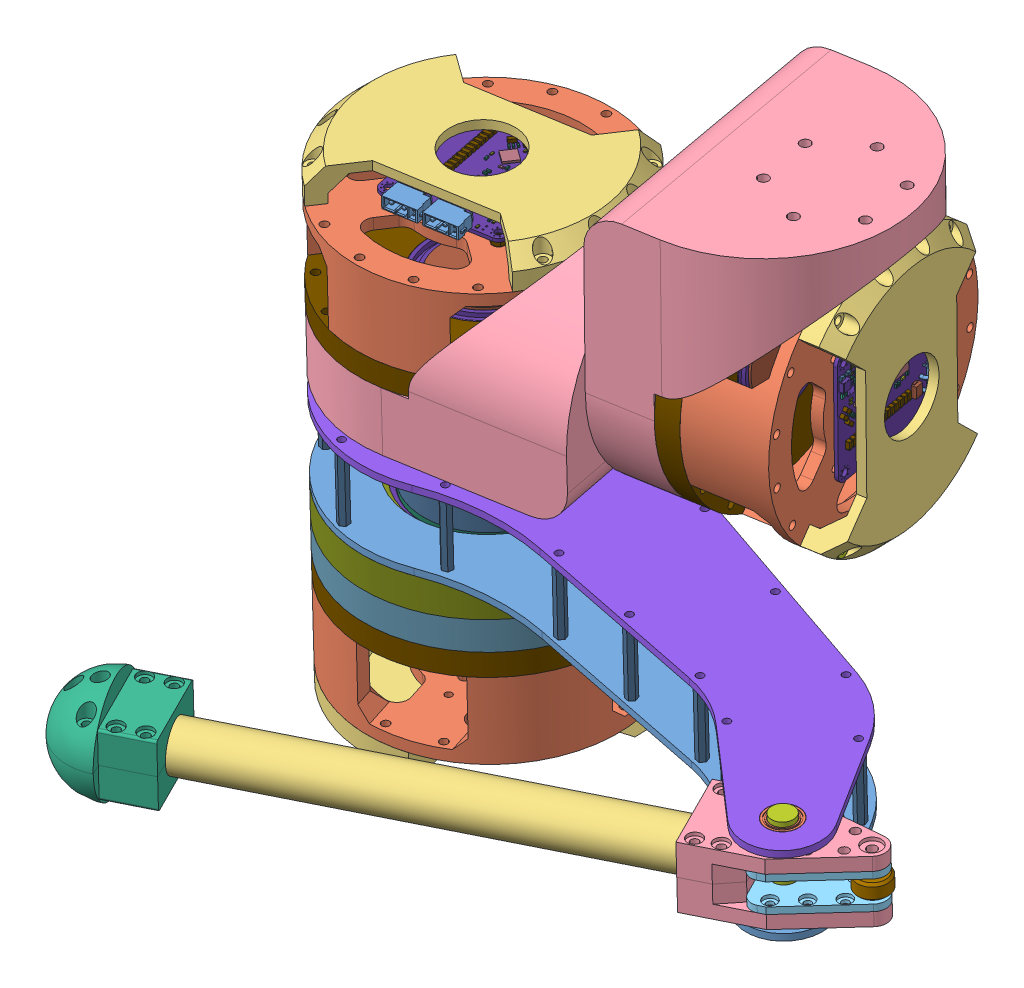
SolidWorks assembly leg, configuration Default. Lengths in mm. (continued)
Components (placement in the parent): (continued)
- Cycloidal _v3-2: Cycloidal _v3 [Default] at (218.9878 344.1312 127.6496) x (0.118839 0.702482 0.701709) z (0.116912 -0.711701 0.692685) size (173.36 87.57 173.15) (continued)
  - radial ball bearing_68_iso-46: radial ball bearing_68_iso [ISO 15 RBB - 1715 - 26,SI,NC,26_68] at (47.6295 89.6575 91.1168) x (-0.000399 1 0) z (0 0 1) size (4 21 21)
  - foc-motor-controller.step-1: foc-motor-controller.step [Default] at (47.4677 32.6574 89.6282) x (0.701413 0.00028 0.712755) z (0.000399 -1 0) size (57.23 50 8.13)
    - RTA0040B.step-1: RTA0040B.step [Default] at (12.5014 -1.6986 1.595) x (-0.707107 -0.707107 0) z (0 0 1) size (6 6 1)
      - FRAME.step-1: FRAME.step [Default] x (1 0 0) z (0 -1 0) size (6 0.2 6)
        - SOLID.step-1: SOLID.step [Default] at origin size (0.4 0.2 0.22)
        - SOLID-0.step-1: SOLID-0.step [Default] at origin size (0.4 0.2 0.22)
        - SOLID-1.step-1: SOLID-1.step [Default] at origin size (0.4 0.2 0.22)
        - SOLID-2.step-1: SOLID-2.step [Default] at origin size (0.4 0.2 0.22)
        - SOLID-3.step-1: SOLID-3.step [Default] at origin size (0.4 0.2 0.22)
        - SOLID-4.step-1: SOLID-4.step [Default] at origin size (0.4 0.2 0.22)
        - SOLID-5.step-1: SOLID-5.step [Default] at origin size (0.4 0.2 0.22)
        - SOLID-6.step-1: SOLID-6.step [Default] at origin size (0.4 0.2 0.22)
        - SOLID-7.step-1: SOLID-7.step [Default] at origin size (0.4 0.2 0.22)
        - SOLID-8.step-1: SOLID-8.step [Default] at origin size (0.4 0.2 0.22)
        - SOLID-9.step-1: SOLID-9.step [Default] at origin size (0.22 0.2 0.4)
        - SOLID-10.step-1: SOLID-10.step [Default] at origin size (0.22 0.2 0.4)
        - SOLID-11.step-1: SOLID-11.step [Default] at origin size (0.22 0.2 0.4)
        - SOLID-12.step-1: SOLID-12.step [Default] at origin size (0.22 0.2 0.4)
        - SOLID-13.step-1: SOLID-13.step [Default] at origin size (0.22 0.2 0.4)
        - SOLID-14.step-1: SOLID-14.step [Default] at origin size (0.22 0.2 0.4)
        - SOLID-15.step-1: SOLID-15.step [Default] at origin size (0.22 0.2 0.4)
        - SOLID-16.step-1: SOLID-16.step [Default] at origin size (0.22 0.2 0.4)
        - SOLID-17.step-1: SOLID-17.step [Default] at origin size (4.15 0.2 4.15)
        - SOLID-18.step-1: SOLID-18.step [Default] at origin size (0.28 0.1 0.28)
        - SOLID-19.step-1: SOLID-19.step [Default] at origin size (0.28 0.1 0.28)
        - SOLID-20.step-1: SOLID-20.step [Default] at origin size (0.28 0.1 0.28)
        - SOLID-21.step-1: SOLID-21.step [Default] at origin size (0.28 0.1 0.28)
        - SOLID-22.step-1: SOLID-22.step [Default] at origin size (0.4 0.2 0.22)
        - SOLID-23.step-1: SOLID-23.step [Default] at origin size (0.4 0.2 0.22)
        - SOLID-24.step-1: SOLID-24.step [Default] at origin size (0.4 0.2 0.22)
        - SOLID-25.step-1: SOLID-25.step [Default] at origin size (0.4 0.2 0.22)
        - SOLID-26.step-1: SOLID-26.step [Default] at origin size (0.4 0.2 0.22)
        - SOLID-27.step-1: SOLID-27.step [Default] at origin size (0.4 0.2 0.22)
        - SOLID-28.step-1: SOLID-28.step [Default] at origin size (0.4 0.2 0.22)
        - SOLID-29.step-1: SOLID-29.step [Default] at origin size (0.4 0.2 0.22)
        - SOLID-30.step-1: SOLID-30.step [Default] at origin size (0.4 0.2 0.22)
        - SOLID-31.step-1: SOLID-31.step [Default] at origin size (0.4 0.2 0.22)
        - SOLID-32.step-1: SOLID-32.step [Default] at origin size (0.22 0.2 0.4)
        - SOLID-33.step-1: SOLID-33.step [Default] at origin size (0.22 0.2 0.4)
        - SOLID-34.step-1: SOLID-34.step [Default] at origin size (0.22 0.2 0.4)
        - SOLID-35.step-1: SOLID-35.step [Default] at origin size (0.22 0.2 0.4)
        - SOLID-36.step-1: SOLID-36.step [Default] at origin size (0.22 0.2 0.4)
        - SOLID-37.step-1: SOLID-37.step [Default] at origin size (0.22 0.2 0.4)
        - SOLID-38.step-1: SOLID-38.step [Default] at origin size (0.22 0.2 0.4)
        - SOLID-39.step-1: SOLID-39.step [Default] at origin size (0.22 0.2 0.4)
        - SOLID-40.step-1: SOLID-40.step [Default] at origin size (0.22 0.2 0.4)
        - SOLID-41.step-1: SOLID-41.step [Default] at origin size (0.22 0.2 0.4)
        - SOLID-42.step-1: SOLID-42.step [Default] at origin size (0.22 0.2 0.4)
        - SOLID-43.step-1: SOLID-43.step [Default] at origin size (0.22 0.2 0.4)
      - BODY.step-1: BODY.step [Default] at (0 0 0.025) x (1 0 0) z (0 -1 0) size (6 0.97 6)
    - Resonator_SMD_Murata_CSTxExxV-3Pin_3.0x1.1mm.step-1: Resonator_SMD_Murata_CSTxExxV-3Pin_3.0x1.1mm.step [Default] at (1.8 -7 1.595) x (0 1 0) z (0 0 1) size (3.2 1.35 0.9)
    - C_0603_1608Metric.step-1: C_0603_1608Metric.step [Default] at (6.2 -16.8 1.595) x (0 -1 0) z (0 0 1) size (1.6 0.8 0.8)
    - R_0603_1608Metric.step-1: R_0603_1608Metric.step [Default] at (11.8 -7.375 1.595) x (0 1 0) z (0 0 1) size (1.6 0.8 0.45)
    - R_0603_1608Metric.step-2: R_0603_1608Metric.step [Default] at (13.8 -16.8 1.595) x (0 1 0) z (0 0 1) size (1.6 0.8 0.45)
    - R_0603_1608Metric.step-3: R_0603_1608Metric.step [Default] at (18.1 -5.36 1.595) size (1.6 0.8 0.45)
    - C_0603_1608Metric.step-2: C_0603_1608Metric.step [Default] at (2.6 -0.5 1.595) x (0 -1 0) z (0 0 1) size (1.6 0.8 0.8)
    - R_0603_1608Metric.step-4: R_0603_1608Metric.step [Default] at (14.6 -11.3 1.595) x (0 1 0) z (0 0 1) size (1.6 0.8 0.45)
    - L_APV_ANR4020.step-1: L_APV_ANR4020.step [Default] at (22.3 -13.7 1.595) x (0 -1 0) z (0 0 1) size (4.02 4 2)
    - C_0603_1608Metric.step-3: C_0603_1608Metric.step [Default] at (0.3 -12.6 1.595) x (-1 0 0) z (0 0 1) size (1.6 0.8 0.8)
    - C_1206_3216Metric.step-1: C_1206_3216Metric.step [Default] at (15.7 11 1.595) x (0 1 0) z (0 0 1) size (3.2 1.6 1.6)
    - C_0603_1608Metric.step-4: C_0603_1608Metric.step [Default] at (0.3 -9.6 1.595) size (1.6 0.8 0.8)
    - R_0603_1608Metric.step-5: R_0603_1608Metric.step [Default] at (12.3 -16.8 1.595) x (0 1 0) z (0 0 1) size (1.6 0.8 0.45)
    - C_0603_1608Metric.step-5: C_0603_1608Metric.step [Default] at (-0.3 -16.6 1.595) x (0 1 0) z (0 0 1) size (1.6 0.8 0.8)
    - R_0603_1608Metric.step-6: R_0603_1608Metric.step [Default] at (10.9 4.1 1.595) size (1.6 0.8 0.45)
    - C_1206_3216Metric.step-2: C_1206_3216Metric.step [Default] at (6.3 11 1.595) x (0 1 0) z (0 0 1) size (3.2 1.6 1.6)
    - XT30PW_2_2_-M.G.B.step-1: XT30PW_2_2_-M.G.B.step [Default] at (-20.5 9.5 1.595) x (0 -1 0) z (-1 0 0) size (15.5 7.1 12.53)
    - R_0603_1608Metric.step-7: R_0603_1608Metric.step [Default] at (0.3 -11.1 1.595) size (1.6 0.8 0.45)
    - C_0603_1608Metric.step-6: C_0603_1608Metric.step [Default] at (19 -0.4 1.595) x (-0.707107 -0.707107 0) z (0 0 1) size (1.6 0.8 0.8)
    - C_1206_3216Metric.step-3: C_1206_3216Metric.step [Default] at (13.3 11 1.595) x (0 1 0) z (0 0 1) size (3.2 1.6 1.6)
    - R_0603_1608Metric.step-8: R_0603_1608Metric.step [Default] at (10.2 -7.375 1.595) x (0 -1 0) z (0 0 1) size (1.6 0.8 0.45)
    - JST_GH_SM08B-GHS-TB_1x08-1MP_P1.25mm_Horizontal.step-1: JST_GH_SM08B-GHS-TB_1x08-1MP_P1.25mm_Horizontal.step [Default] at (10 -22 1.595) size (13.25 4.95 4.25)
    - C_1206_3216Metric.step-4: C_1206_3216Metric.step [Default] at (-12.3 11 1.595) x (0 1 0) z (0 0 1) size (3.2 1.6 1.6)
    - JST_GH_SM06B-GHS-TB_1x06-1MP_P1.25mm_Horizontal.step-1: JST_GH_SM06B-GHS-TB_1x06-1MP_P1.25mm_Horizontal.step [Default] at (-4.3 -22 1.595) size (10.75 4.95 4.25)
    - C_0603_1608Metric.step-7: C_0603_1608Metric.step [Default] at (7.3 -4.5 1.595) x (-1 0 0) z (0 0 1) size (1.6 0.8 0.8)
    - R_0603_1608Metric.step-9: R_0603_1608Metric.step [Default] at (18.1 -3.86 1.595) x (-1 0 0) z (0 0 1) size (1.6 0.8 0.45)
    - C_1206_3216Metric.step-5: C_1206_3216Metric.step [Default] at (22.6794 -1.2206 1.595) x (0.707107 -0.707107 0) z (0 0 1) size (3.2 1.6 1.6)
    - R_Array_Convex_4x0402.step-1: R_Array_Convex_4x0402.step [Default] at (6.8 -2.5 1.595) size (1 2 0.35)
    - R_0603_1608Metric.step-10: R_0603_1608Metric.step [Default] at (7.7 -16.8 1.595) x (0 -1 0) z (0 0 1) size (1.6 0.8 0.45)
    - C_1206_3216Metric.step-6: C_1206_3216Metric.step [Default] at (8.7 11 1.595) x (0 1 0) z (0 0 1) size (3.2 1.6 1.6)
    - C_0603_1608Metric.step-8: C_0603_1608Metric.step [Default] at (16.1 -11.3 1.595) x (0 1 0) z (0 0 1) size (1.6 0.8 0.8)
    - SOT-23-5.step-1: SOT-23-5.step [Default] at (-3.1 -16.6 1.595) x (-1 0 0) z (0 0 1) size (2.8 2.9 1.55)
    - C_0603_1608Metric.step-9: C_0603_1608Metric.step [Default] at (17.8 -13.6 1.595) size (1.6 0.8 0.8)
    - R_0603_1608Metric.step-11: R_0603_1608Metric.step [Default] at (-11.5 -20.3875 1.595) x (0 -1 0) z (0 0 1) size (1.6 0.8 0.45)
    - C_0603_1608Metric.step-10: C_0603_1608Metric.step [Default] at (-12.4 2.3 1.595) x (0 1 0) z (0 0 1) size (1.6 0.8 0.8)
    - C_1206_3216Metric.step-7: C_1206_3216Metric.step [Default] at (18 11 1.595) x (0 1 0) z (0 0 1) size (3.2 1.6 1.6)
    - R_0603_1608Metric.step-12: R_0603_1608Metric.step [Default] at (-10.8105 -14.9971 1.595) x (-1 0 0) z (0 0 1) size (1.6 0.8 0.45)
    - C_0603_1608Metric.step-11: C_0603_1608Metric.step [Default] at (-13.8 -9.4 1.595) x (-1 0 0) z (0 0 1) size (1.6 0.8 0.8)
    - R_0603_1608Metric.step-13: R_0603_1608Metric.step [Default] at (-23.15 -14.5 1.595) x (-1 0 0) z (0 0 1) size (1.6 0.8 0.45)
    - C_0603_1608Metric.step-12: C_0603_1608Metric.step [Default] at (1.1 -0.2 1.595) x (0 1 0) z (0 0 1) size (1.6 0.8 0.8)
    - D_0805_2012Metric.step-1: D_0805_2012Metric.step [Default] at (22.9 -9.6 1.595) x (0 1 0) z (0 0 1) size (2 1.27 0.8)
    - C_0603_1608Metric.step-13: C_0603_1608Metric.step [Default] at (-7.8 3.775 1.595) x (0 -1 0) z (0 0 1) size (1.6 0.8 0.8)
    - R_0603_1608Metric.step-14: R_0603_1608Metric.step [Default] at (-6.4 -12.825 1.595) x (0 1 0) z (0 0 1) size (1.6 0.8 0.45)
    - L_0603_1608Metric.step-1: L_0603_1608Metric.step [Default] at (-10.1 3 1.595) size (1.6 0.8 0.8)
    - C_0603_1608Metric.step-14: C_0603_1608Metric.step [Default] at (17.9 0.7 1.595) x (-0.707107 -0.707107 0) z (0 0 1) size (1.6 0.8 0.8)
    - HVSSOP-10.step-1: HVSSOP-10.step [Default] at (18.6 -9.6 1.595) x (0 -1 0) z (-1 0 0) size (4.9 1.1 3)
    - C_0603_1608Metric.step-15: C_0603_1608Metric.step [Default] at (7.9 4.1 1.595) x (-1 0 0) z (0 0 1) size (1.6 0.8 0.8)
    - C_0603_1608Metric.step-16: C_0603_1608Metric.step [Default] at (21.1 -9.6 1.595) x (0 -1 0) z (0 0 1) size (1.6 0.8 0.8)
    - R_0603_1608Metric.step-15: R_0603_1608Metric.step [Default] at (-10.8105 -11.9971 1.595) x (-1 0 0) z (0 0 1) size (1.6 0.8 0.45)
    - R_0603_1608Metric.step-16: R_0603_1608Metric.step [Default] at (-18.2 -17.4 1.595) size (1.6 0.8 0.45)
    - C_1206_3216Metric.step-8: C_1206_3216Metric.step [Default] at (-3 11 1.595) x (0 1 0) z (0 0 1) size (3.2 1.6 1.6)
    - R_0603_1608Metric.step-17: R_0603_1608Metric.step [Default] at (-16.9 -20.4 1.595) x (0 -1 0) z (0 0 1) size (1.6 0.8 0.45)
    - R_0603_1608Metric.step-18: R_0603_1608Metric.step [Default] at (-13.3 -20.3875 1.595) x (0 -1 0) z (0 0 1) size (1.6 0.8 0.45)
    - R_0603_1608Metric.step-19: R_0603_1608Metric.step [Default] at (-15.1 -20.3875 1.595) x (0 -1 0) z (0 0 1) size (1.6 0.8 0.45)
    - C_0603_1608Metric.step-17: C_0603_1608Metric.step [Default] at (15.5 -14.4 1.595) x (0 -1 0) z (0 0 1) size (1.6 0.8 0.8)
    - LED_0603_1608Metric.step-1: LED_0603_1608Metric.step [Default] at (-11.5 -23.3875 1.595) x (0 1 0) z (0 0 1) size (1.6 0.8 1.1)
    - C_0805_2012Metric.step-1: C_0805_2012Metric.step [Default] at (19.95 -17 1.595) size (2 1.25 1.25)
    - D_SMB.step-1: D_SMB.step [Default] at (-16.5 11.208 1.595) x (0 -1 0) z (0 0 1) size (5.3 3.55 2.15)
    - C_1206_3216Metric.step-9: C_1206_3216Metric.step [Default] at (-5.3 11 1.595) x (0 1 0) z (0 0 1) size (3.2 1.6 1.6)
    - XT30PW_2_2_-M.G.B.step-2: XT30PW_2_2_-M.G.B.step [Default] at (-20.5 -6.5 1.595) x (0 -1 0) z (-1 0 0) size (15.5 7.1 12.53)
    - C_1206_3216Metric.step-10: C_1206_3216Metric.step [Default] at (1.7 11 1.595) x (0 1 0) z (0 0 1) size (3.2 1.6 1.6)
    - C_1206_3216Metric.step-11: C_1206_3216Metric.step [Default] at (11 11 1.595) x (0 1 0) z (0 0 1) size (3.2 1.6 1.6)
    - C_0603_1608Metric.step-18: C_0603_1608Metric.step [Default] at (-6.3 3.775 1.595) x (0 -1 0) z (0 0 1) size (1.6 0.8 0.8)
    - C_0603_1608Metric.step-19: C_0603_1608Metric.step [Default] at (16.8686 1.7314 1.595) x (0.707107 0.707107 0) z (0 0 1) size (1.6 0.8 0.8)
    - C_0603_1608Metric.step-20: C_0603_1608Metric.step [Default] at (-15.0105 -11.1 1.595) size (1.6 0.8 0.8)
    - C_1206_3216Metric.step-12: C_1206_3216Metric.step [Default] at (-7.7 11 1.595) x (0 1 0) z (0 0 1) size (3.2 1.6 1.6)
    - C_0603_1608Metric.step-21: C_0603_1608Metric.step [Default] at (-18.2 -15.8 1.595) size (1.6 0.8 0.8)
    - C_0603_1608Metric.step-22: C_0603_1608Metric.step [Default] at (-2.1 -11.3 1.595) x (0 -1 0) z (0 0 1) size (1.6 0.8 0.8)
    - C_0603_1608Metric.step-23: C_0603_1608Metric.step [Default] at (-10.8105 -13.4971 1.595) size (1.6 0.8 0.8)
    - C_1206_3216Metric.step-13: C_1206_3216Metric.step [Default] at (4 11 1.595) x (0 1 0) z (0 0 1) size (3.2 1.6 1.6)
    - R_0603_1608Metric.step-20: R_0603_1608Metric.step [Default] at (16 -17.8 1.595) x (0 1 0) z (0 0 1) size (1.6 0.8 0.45)
    - Texas_S-PVSON-N8.step-1: Texas_S-PVSON-N8.step [Default] at (-14.4105 -13.7 1.595) x (-1 0 0) z (0 0 1) size (3 2.98 0.92)
    - C_1206_3216Metric.step-14: C_1206_3216Metric.step [Default] at (21 -2.9 1.595) x (0.707107 -0.707107 0) z (0 0 1) size (3.2 1.6 1.6)
    - C_0603_1608Metric.step-24: C_0603_1608Metric.step [Default] at (-5.9 -16.6 1.595) x (0 1 0) z (0 0 1) size (1.6 0.8 0.8)
    - C_0603_1608Metric.step-25: C_0603_1608Metric.step [Default] at (-3.1 -14.1 1.595) size (1.6 0.8 0.8)
    - R_0603_1608Metric.step-21: R_0603_1608Metric.step [Default] at (7.2 -7.375 1.595) x (0 -1 0) z (0 0 1) size (1.6 0.8 0.45)
    - C_1206_3216Metric.step-15: C_1206_3216Metric.step [Default] at (-0.7 11 1.595) x (0 1 0) z (0 0 1) size (3.2 1.6 1.6)
    - LQFP-64_10x10mm_P0.5mm.step-1: LQFP-64_10x10mm_P0.5mm.step [Default] at (-7 -4.5 1.595) x (-1 0 0) z (0 0 1) size (12 12 1.5)
    - C_0805_2012Metric.step-2: C_0805_2012Metric.step [Default] at (23.35 -17 1.595) x (-1 0 0) z (0 0 1) size (2 1.25 1.25)
    - C_0603_1608Metric.step-26: C_0603_1608Metric.step [Default] at (10.8 -16.8 1.595) x (0 -1 0) z (0 0 1) size (1.6 0.8 0.8)
    - R_0603_1608Metric.step-22: R_0603_1608Metric.step [Default] at (17.5 -17.8 1.595) x (0 -1 0) z (0 0 1) size (1.6 0.8 0.45)
    - C_1206_3216Metric.step-16: C_1206_3216Metric.step [Default] at (20.3 11 1.595) x (0 1 0) z (0 0 1) size (3.2 1.6 1.6)
    - R_0603_1608Metric.step-23: R_0603_1608Metric.step [Default] at (9.2 -16.8 1.595) x (0 -1 0) z (0 0 1) size (1.6 0.8 0.45)
    - C_1206_3216Metric.step-17: C_1206_3216Metric.step [Default] at (-10 11 1.595) x (0 1 0) z (0 0 1) size (3.2 1.6 1.6)
    - R_0603_1608Metric.step-24: R_0603_1608Metric.step [Default] at (17.8 -15.2 1.595) size (1.6 0.8 0.45)
    - C_1206_3216Metric.step-18: C_1206_3216Metric.step [Default] at (19.9 2.6 1.595) x (-0.707107 0.707107 0) z (0 0 1) size (3.2 1.6 1.6)
    - C_0603_1608Metric.step-27: C_0603_1608Metric.step [Default] at (13.4 -7.375 1.595) x (0 -1 0) z (0 0 1) size (1.6 0.8 0.8)
    - R_0603_1608Metric.step-25: R_0603_1608Metric.step [Default] at (8.7 -7.375 1.595) x (0 -1 0) z (0 0 1) size (1.6 0.8 0.45)
    - PQFN-8-EP_6x5mm_P1.27mm_Generic.step-1: PQFN-8-EP_6x5mm_P1.27mm_Generic.step [Default] at (4.9 14.4 -0.085) x (0 1 0) z (0 0 -1) size (6.15 5.15 1.09)
    - C_0805_2012Metric.step-3: C_0805_2012Metric.step [Default] at (-3 8.9 -0.085) x (0 1 0) z (0 0 -1) size (2 1.25 1.25)
    - C_0603_1608Metric.step-28: C_0603_1608Metric.step [Default] at (1.5 -4.3 -0.085) x (0 1 0) z (0 0 -1) size (1.6 0.8 0.8)
    - R_2512_6332Metric.step-1: R_2512_6332Metric.step [Default] at (2.1 8.6 -0.085) x (-1 0 0) z (0 0 -1) size (6.3 3.2 0.6)
    - C_0805_2012Metric.step-4: C_0805_2012Metric.step [Default] at (18.8 8.9 -0.085) x (0 1 0) z (0 0 -1) size (2 1.25 1.25)
    - C_0805_2012Metric.step-5: C_0805_2012Metric.step [Default] at (-5.2 8.901 -0.085) x (0 1 0) z (0 0 -1) size (2 1.25 1.25)
    - PQFN-8-EP_6x5mm_P1.27mm_Generic.step-2: PQFN-8-EP_6x5mm_P1.27mm_Generic.step [Default] at (16.9 14.6 -0.085) x (0 -1 0) z (0 0 -1) size (6.15 5.15 1.09)
    - PQFN-8-EP_6x5mm_P1.27mm_Generic.step-3: PQFN-8-EP_6x5mm_P1.27mm_Generic.step [Default] at (-1.1 14.6 -0.085) x (0 -1 0) z (0 0 -1) size (6.15 5.15 1.09)
    - R_0603_1608Metric.step-26: R_0603_1608Metric.step [Default] at (8.2 8.8 -0.085) x (0 1 0) z (0 0 -1) size (1.6 0.8 0.45)
    - R_2512_6332Metric.step-2: R_2512_6332Metric.step [Default] at (-10.3 8.601 -0.085) x (1 0 0) z (0 0 -1) size (6.3 3.2 0.6)
    - TSSOP-16_4.4x5mm_P0.65mm.step-1: TSSOP-16_4.4x5mm_P0.65mm.step [Default] at (0 0 -0.085) x (-1 0 0) z (0 0 -1) size (6.4 5 1.1)
    - C_0603_1608Metric.step-29: C_0603_1608Metric.step [Default] at (0 -4.25 -0.085) x (0 1 0) z (0 0 -1) size (1.6 0.8 0.8)
    - PQFN-8-EP_6x5mm_P1.27mm_Generic.step-4: PQFN-8-EP_6x5mm_P1.27mm_Generic.step [Default] at (10.9 14.4 -0.085) x (0 1 0) z (0 0 -1) size (6.15 5.15 1.09)
    - R_2512_6332Metric.step-3: R_2512_6332Metric.step [Default] at (13.7 8.6 -0.085) x (1 0 0) z (0 0 -1) size (6.3 3.2 0.6)
    - PQFN-8-EP_6x5mm_P1.27mm_Generic.step-5: PQFN-8-EP_6x5mm_P1.27mm_Generic.step [Default] at (-13.1 14.401 -0.085) x (0 1 0) z (0 0 -1) size (6.15 5.15 1.09)
    - C_0603_1608Metric.step-30: C_0603_1608Metric.step [Default] at (-1.5 -4.3 -0.085) x (0 -1 0) z (0 0 -1) size (1.6 0.8 0.8)
    - PQFN-8-EP_6x5mm_P1.27mm_Generic.step-6: PQFN-8-EP_6x5mm_P1.27mm_Generic.step [Default] at (-7.1 14.601 -0.085) x (0 -1 0) z (0 0 -1) size (6.15 5.15 1.09)
    - foc-motor-controller_PCB.step-1: foc-motor-controller_PCB.step [Default] at origin size (50 50 1.51)
  - hex nut style 1 gradeab_iso-1: hex nut style 1 gradeab_iso [ISO - 4032 - M3 - W - N] at (47.7115 32.6575 59.2236) x (1 0.000399 0) z (0.000399 -1 0) size (5.5 6.35 2.4)
  - Cycloidal_Discs_8308-1: Cycloidal_Discs_8308 [Default] at (-11.9184 124.164 51.5043) x (0.028527 0.000011 0.999593) z (0.999593 0.000399 -0.028527) size (79.25 5 79.73)
    - Cycloidal_Discs-1: Cycloidal_Discs [Default] at (38.3081 39.5303 58.0959) size (79.25 5 79.73)
  - Cycloidal_Discs_8308-2: Cycloidal_Discs_8308 [Default] at (62.1667 47.133 159.1742) x (-0.931329 -0.000371 -0.364178) z (0.364178 0.000145 -0.931329) size (79.25 5 79.73)
    - Cycloidal_Discs-1: Cycloidal_Discs [Default] at (38.3081 39.5303 58.0959) size (79.25 5 79.73)
  - Motor_Cover_v2-2: Motor_Cover_v2 [Default] at (47.4667 35.0574 89.6282) x (0.999968 0.000399 0.00802) z (-0.00802 -0.000003 0.999968) size (115 34.6 115)
  - driver_cover-1: driver_cover [Default] at (47.4667 35.0574 89.6282) x (0.702656 0.00028 0.711529) z (0.711529 0.000284 -0.702656) size (81.32 15 115)
  - Cover_new-1: Cover_new [Default] at (47.4437 92.6574 89.6282) x (0.701413 0.00028 0.712755) z (-0.712755 -0.000284 0.701413) size (115 87.5 130)
  - Output_Shaft-2: Output_Shaft [Default] at (47.4437 92.6574 89.6282) x (0.572675 0.000228 0.819783) z (-0.819783 -0.000327 0.572675) size (70 14 70)
  - radial ball bearing_68_iso-47: radial ball bearing_68_iso [ISO 15 RBB - 289 - 14,SI,NC,14_68] at (61.9924 89.1632 109.081) x (0.000399 -1 0) z (-0.055662 -0.000022 0.99845) size (5 17 17)
  - radial ball bearing_68_iso-48: radial ball bearing_68_iso [ISO 15 RBB - 289 - 14,SI,NC,14_68] at (59.3269 82.1622 107.722) x (0.000399 -1 0) z (-0.055662 -0.000022 0.99845) size (5 17 17)
  - m4x14-1: m4x14 [Default] at (47.0925 68.4573 134.6267) x (0.999623 0.000399 0.027466) z (-0.027466 -0.000011 0.999623) size (8 15.2 8)
  - M3x20-1: M3x20 [Default] at (43.4726 96.3558 90.1203) x (-0.837193 -0.000334 -0.546908) z (-0.546908 -0.000218 0.837193) size (6 21.2 6)
  - M3x10-1: M3x10 [Default] at (36.5111 25.853 142.5044) x (0.424034 0.000169 -0.905646) z (0.905646 0.000361 0.424034) size (6 11.2 6)
  - m3x60-1: m3x60 [Default] at (17.1068 35.0453 134.2855) x (-0.837193 -0.000334 -0.546908) z (-0.546908 -0.000218 0.837193) size (5.3 63 5.3)
  - m6-1: m6 [Default] at (60.6129 98.6627 108.4832) x (-0.153131 -0.000061 0.988206) z (0.988206 0.000394 0.153131) size (6 16 6)
- Output_2-2: Output_2 [Default] at (129.939 313.6971 240.802) x (0.005689 0.999416 0.033707) z (0.166329 -0.034184 0.985478) size (60 8 60)
Mates (geometry in assembly coordinates):
- Concentric2: concentric anti-aligned: cylinder of Leg_Upper - Copy-1 through (280.1682 210.6635 348.3638) axis (-0.005682 -0.999417 -0.033664) radius 7.5; cylinder of Bearing_10x15x4-1 through (280.1512 207.6652 348.2628) axis (0.005682 0.999417 0.033664) radius 5
- Coincident2: coincident aligned: plane of Leg_Upper - Copy-1 through (49.985 212.2572 250.7825) normal (-0.005682 -0.999417 -0.033664); plane of Bearing_10x15x4-1 through (280.1512 207.6652 348.2628) normal (-0.005682 -0.999417 -0.033664)
- Concentric3: concentric aligned: cylinder of Bearing_10x15x4-1 through (280.1512 207.6652 348.2628) axis (0.005682 0.999417 0.033664) radius 5; cylinder of Leg_lower-1/m10-1 through (280.1398 205.6664 348.1955) axis (0.005682 0.999417 0.033664) radius 5
- Coincident3: coincident anti-aligned: plane of Bearing_10x15x4-1 through (280.1739 211.6629 348.3975) normal (0.005682 0.999417 0.033664); plane of Leg_lower-1/knee-1 through (280.1739 211.6629 348.3975) normal (-0.005682 -0.999417 -0.033664)
- Concentric41: concentric anti-aligned: cylinder of Leg_Upper-1 through (280.3557 243.6442 349.4747) axis (-0.005682 -0.999417 -0.033664) radius 7.5; cylinder of Bearing_10x15x4-2 through (280.3529 243.1445 349.4579) axis (0.005682 0.999417 0.033664) radius 6.5
- Coincident41: coincident aligned: plane of Leg_Upper-1 through (50.1895 248.2362 251.9944) normal (0.005682 0.999417 0.033664); plane of Bearing_10x15x4-2 through (280.3557 243.6442 349.4747) normal (0.005682 0.999417 0.033664)
- Concentric5: concentric aligned: cylinder of Leg_Upper - Copy-1 through (50.002 215.2555 250.8835) axis (-0.005682 -0.999417 -0.033664) radius 57.5; cylinder of Leg_Upper-1 through (50.1895 248.2362 251.9944) axis (-0.005682 -0.999417 -0.033664) radius 57.5
- Concentric6: concentric anti-aligned: cylinder of Leg_lower-1/m10-1 through (280.1398 205.6664 348.1955) axis (0.005682 0.999417 0.033664) radius 5; cylinder of Bearing_10x15x4-2 through (280.3557 243.6442 349.4747) axis (-0.005682 -0.999417 -0.033664) radius 5
- Coincident6: coincident anti-aligned: plane of Leg_lower-1/knee-3 through (280.333 239.6466 349.3401) normal (0.005682 0.999417 0.033664); plane of Bearing_10x15x4-2 through (280.333 239.6466 349.3401) normal (-0.005682 -0.999417 -0.033664)
- Concentric7: concentric aligned: cylinder of Leg_lower-1/knee - Copy-1 through (307.2468 220.9429 335.6719) axis (-0.005682 -0.999417 -0.033664) radius 2.1; cylinder of Link_Rod-1 through (307.2951 229.4379 335.9581) axis (-0.005682 -0.999417 -0.033664) radius 2
- Coincident7: coincident aligned: plane of Leg_lower-1/Cacbon_20x18x200-1 through (77.5901 223.5155 446.5825) normal (-0.005682 -0.999417 -0.033664); plane of Link_Rod-1 through (59.5022 231.363 216.6593) normal (-0.005682 -0.999417 -0.033664)
- Concentric42: concentric anti-aligned: cylinder of Leg_Upper - Copy-1 through (49.9452 205.2613 250.5468) axis (0.005682 0.999417 0.033664) radius 35; cylinder of Link_rod_2-1 through (50.0673 226.7488 251.2706) axis (-0.005682 -0.999417 -0.033664) radius 30
- Concentric43: concentric aligned: cylinder of Link_Rod-1 through (59.5221 234.861 216.7771) axis (-0.005682 -0.999417 -0.033664) radius 2; cylinder of Link_rod_2-1 through (59.4823 227.8651 216.5415) axis (-0.005682 -0.999417 -0.033664) radius 2.5
- Concentric44: concentric aligned: cylinder of Leg_Upper - Copy-1 through (50.002 215.2555 250.8835) axis (-0.005682 -0.999417 -0.033664) radius 57.5; cylinder of Cycloidal-1/Cover-1 through (49.9736 210.2584 250.7151) axis (-0.005682 -0.999417 -0.033664) radius 57.5
- Coincident44: coincident anti-aligned: plane of Leg_Upper - Copy-1 through (49.985 212.2572 250.7825) normal (-0.005682 -0.999417 -0.033664); plane of Cycloidal-1/Cover-1 through (49.985 212.2572 250.7825) normal (0.005682 0.999417 0.033664)
- Coincident45: coincident anti-aligned: plane of Link_rod_2-1 through (49.985 212.2572 250.7825) normal (-0.005682 -0.999417 -0.033664); plane of Cycloidal-1/Output_Shaft-1 through (49.985 212.2572 250.7825) normal (0.005682 0.999417 0.033664)
- Coincident46: coincident anti-aligned: plane of Leg_Upper-1 through (50.1895 248.2362 251.9944) normal (0.005682 0.999417 0.033664); plane of Output_2-1 through (50.1896 248.2362 251.9954) normal (-0.005682 -0.999417 -0.033664)
- Concentric46: concentric anti-aligned: cylinder of Leg_Upper-1 through (59.1667 248.8981 230.829) axis (-0.005682 -0.999417 -0.033664) radius 2; cylinder of Output_2-1 through (59.1667 248.8981 230.829) axis (0.005682 0.999417 0.033664) radius 2.1
- Concentric47: concentric anti-aligned: cylinder of Leg_Upper-1 through (41.2123 247.5744 273.1597) axis (-0.005682 -0.999417 -0.033664) radius 2; cylinder of Output_2-1 through (41.2123 247.5744 273.1597) axis (0.005682 0.999417 0.033664) radius 2.1
- Coincident47: coincident anti-aligned: plane of Cycloidal _v3-1/Output_Shaft-2 through (50.235 256.2316 252.2637) normal (-0.005682 -0.999417 -0.033664); plane of Output_2-1 through (50.2351 256.2315 252.2647) normal (0.005682 0.999417 0.033664)
- Concentric48: concentric aligned: cylinder of Cycloidal _v3-1/Output_Shaft-2 through (50.235 256.2316 252.2637) axis (0.005682 0.999417 0.033664) radius 30; cylinder of Output_2-1 through (50.1896 248.2362 251.9954) axis (0.005682 0.999417 0.033664) radius 30
- Concentric49: concentric aligned: cylinder of Leg_Upper-1 through (3.6267 247.58 279.3344) axis (-0.005682 -0.999417 -0.033664) radius 1.6; cylinder of Brass_m3-1 through (3.6097 244.5818 279.2334) axis (-0.005682 -0.999417 -0.033664) radius 1.5
- Coincident48: coincident anti-aligned: plane of Leg_Upper-1 through (50.1725 245.238 251.8934) normal (-0.005682 -0.999417 -0.033664); plane of Brass_m3-1 through (3.6097 244.5818 279.2334) normal (0.005682 0.999417 0.033664)
- Concentric50: concentric anti-aligned: circle of Leg_Upper-1; cylinder of Brass_m3-11 through (207.9138 242.2445 314.1411) axis (-0.005682 -0.999417 -0.033664) radius 1.5
- Concentric51: concentric anti-aligned: circle of Leg_Upper-1; cylinder of Brass_m3-12 through (241.3192 243.1417 281.8674) axis (-0.005682 -0.999417 -0.033664) radius 1.5
- Concentric52: concentric anti-aligned: cylinder of Leg_Upper-1 through (231.1654 234.7364 325.1803) axis (0.005682 0.999417 0.033664) radius 1.6; cylinder of Brass_m3-9 through (231.2052 241.7323 325.416) axis (-0.005682 -0.999417 -0.033664) radius 1.5
- Concentric53: concentric anti-aligned: circle of Leg_Upper-1; cylinder of Brass_m3-10 through (268.1609 242.2757 303.0465) axis (-0.005682 -0.999417 -0.033664) radius 1.5
- Coincident49: coincident anti-aligned: plane of Leg_Upper-1 through (50.1725 245.238 251.8934) normal (-0.005682 -0.999417 -0.033664); plane of Brass_m3-11 through (207.9138 242.2445 314.1411) normal (0.005682 0.999417 0.033664)
- Coincident50: coincident anti-aligned: plane of Leg_Upper-1 through (50.1725 245.238 251.8934) normal (-0.005682 -0.999417 -0.033664); plane of Brass_m3-9 through (231.2052 241.7323 325.416) normal (0.005682 0.999417 0.033664)
- Coincident51: coincident anti-aligned: plane of Leg_Upper-1 through (50.1725 245.238 251.8934) normal (-0.005682 -0.999417 -0.033664); circle of Brass_m3-10
- Coincident52: coincident anti-aligned: plane of Leg_Upper-1 through (50.1725 245.238 251.8934) normal (-0.005682 -0.999417 -0.033664); plane of Brass_m3-12 through (241.3192 243.1417 281.8674) normal (0.005682 0.999417 0.033664)
- Coincident53: coincident aligned: plane of Leg_Upper - Copy-1 through (49.985 212.2572 250.7825) normal (-0.005682 -0.999417 -0.033664); plane of Link_rod_2-1 through (49.985 212.2572 250.7825) normal (-0.005682 -0.999417 -0.033664)
- Coincident54: coincident anti-aligned: plane of Cycloidal _v3-1/Cover_new-1 through (112.2394 272.1865 184.004) normal (0.986054 0 -0.166427); plane of Output_2-2 through (122.0506 313.6971 242.1334) normal (-0.986054 0 0.166427)
- Coincident55: coincident aligned: axis of Cycloidal _v3-1/Cover_new-1 through (108.3644 314.4833 221.1317) axis (0.986054 0 -0.166427); line of Output_2-2 through (118.225 314.4833 219.4674) axis (0.986054 0 -0.166427)
- Concentric54: concentric aligned: line of Cycloidal _v3-1/Cover_new-1 through (116.0156 312.9128 266.4637) axis (0.986054 0 -0.166427); cylinder of Output_2-2 through (125.8761 312.9128 264.7994) axis (0.986054 0 -0.166427) radius 2.1
- Coincident56: coincident anti-aligned: plane of Cycloidal _v3-2/Output_Shaft-2 through (129.939 313.6971 240.802) normal (-0.986054 0 0.166427); plane of Output_2-2 through (129.939 313.6971 240.802) normal (0.986054 0 -0.166427)
- Concentric55: concentric aligned: cylinder of Output_2-2 through (122.0506 313.6971 242.1334) axis (0.986054 0 -0.166427) radius 30; cylinder of Cycloidal _v3-2/Cover_new-1 through (129.939 313.6971 240.802) axis (0.986054 0 -0.166427) radius 57.5
